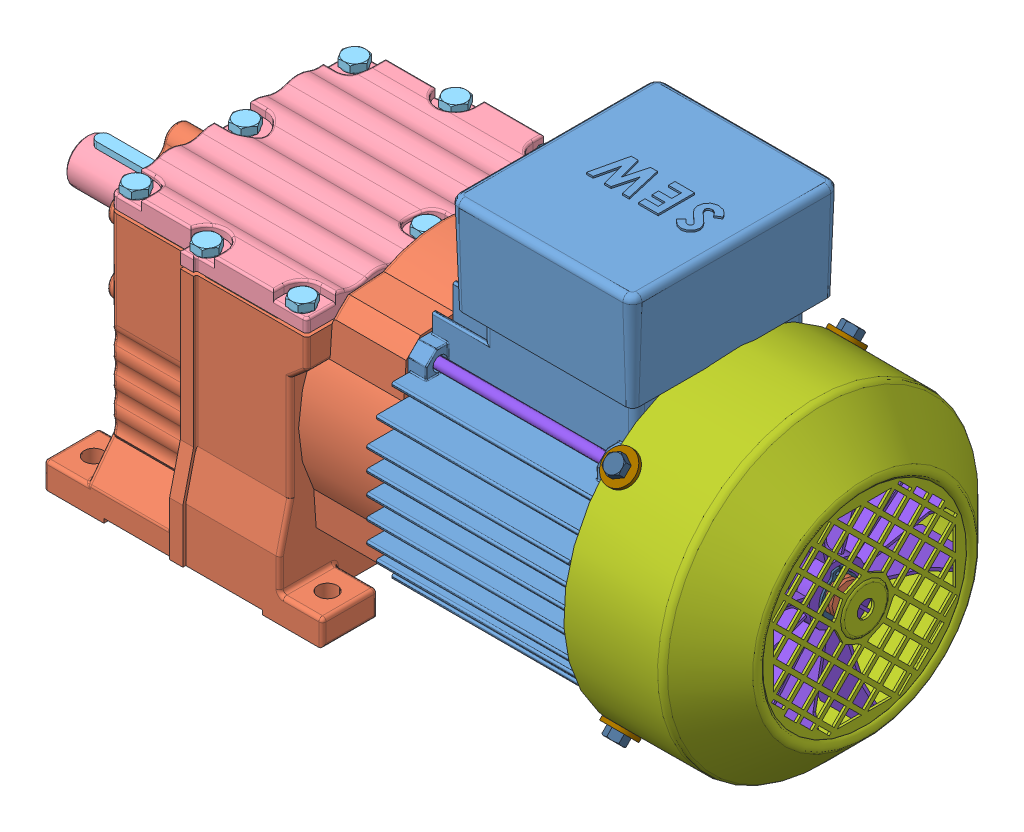
SolidWorks assembly motoreducteur_sew, configuration normale. Lengths in mm.
Overall size (364.24 223.98 208.79).
70 component instances, 46 part files, 12 mates.
Components (placement in the parent):
- bati-1: bati [Défaut] at (-5.3482 -13.3943 0) size (322.68 223.98 208.79)
  - stator-1: stator [Défaut] at origin size (109 189.98 140.8)
  - carter_reducteur-1: carter_reducteur [Défaut] at (-128.4692 42 0) x (0 0 1) z (0 1 0) size (138.68 158.48 134.18)
  - joint plat-1: joint plat [Défaut] at (-128.4692 43.6 0.18) x (0 0 -1) z (0 -1 0) size (123.38 94.6 1.6)
  - couvercle-1: couvercle [Défaut] at (-128.4692 43.6 0) x (0 0 1) z (0 1 0) size (128.68 97.78 10)
  - vis HM6-16-1: vis HM6-16 [Default] at (-122.22 53.6 -51) x (0 -1 0) z (0 0 1) size (20 11.55 10)
  - vis HM6-16-4: vis HM6-16 [Default] at (-122.22 53.6 0) x (0 -1 0) z (0 0 1) size (20 11.55 10)
  - vis HM6-16-5: vis HM6-16 [Default] at (-122.22 53.6 51) x (0 -1 0) z (0 0 1) size (20 11.55 10)
  - vis HM6-16-6: vis HM6-16 [Default] at (-37.62 53.6 58) x (0 -1 0) z (0 0 1) size (20 11.55 10)
  - vis HM6-16-7: vis HM6-16 [Default] at (-37.62 53.6 0) x (0 -1 0) z (0 0 1) size (20 11.55 10)
  - vis HM6-16-8: vis HM6-16 [Default] at (-37.62 53.6 -58) x (0 -1 0) z (0 0 1) size (20 11.55 10)
  - vis HM6-16-9: vis HM6-16 [Default] at (-82.22 53.6 58) x (0 -1 0) z (0 0 1) size (20 11.55 10)
  - vis HM6-16-10: vis HM6-16 [Default] at (-82.22 53.6 -58) x (0 -1 0) z (0 0 1) size (20 11.55 10)
  - flasque-1: flasque [Défaut] at (127.08 0 0) x (-1 0 0) z (0 -0.707107 -0.707107) size (27.7 143 143)
  - carter-1: carter [Défaut] at (166.08 0 0) x (1 0 0) z (0 0.707107 0.707107) size (67.9 147.64 147.64)
  - vis Chc - M5 x 115-15-1: vis Chc - M5 x 115-15 [Default] at (113.58 43.5578 -43.5578) x (-1 0 0) z (0 -0.707107 0.707107) size (118.5 9.24 8)
  - vis Chc - M5 x 115-15-2: vis Chc - M5 x 115-15 [Default] at (113.58 -43.5578 -43.5578) x (-1 0 0) z (0 0.707107 0.707107) size (118.5 9.24 8)
  - vis Chc - M5 x 115-15-3: vis Chc - M5 x 115-15 [Default] at (113.58 -43.5578 43.5578) x (-1 0 0) z (0 0.707107 -0.707107) size (118.5 9.24 8)
  - vis Chc - M5 x 115-15-4: vis Chc - M5 x 115-15 [Default] at (113.58 43.5578 43.5578) x (-1 0 0) z (0 -0.707107 -0.707107) size (118.5 9.24 8)
  - rondelle M5-1: rondelle M5 [Default] at (105.58 52.1986 52.1986) x (0 -0.707107 -0.707107) z (0.685439 -0.514866 0.514866) size (1.75 15 15)
  - vis HM5-6-1: vis HM5-6 [Default] at (105.58 56.1231 56.1231) x (0 -0.707107 -0.707107) z (0.5 -0.612372 0.612372) size (9.8 9.24 8)
  - vis HM5-6-2: vis HM5-6 [Default] at (105.58 -56.1231 56.1231) x (0 0.707107 -0.707107) z (0.5 -0.612372 -0.612372) size (9.8 9.24 8)
  - vis HM5-6-3: vis HM5-6 [Default] at (105.58 -56.1231 -56.1231) x (0 0.707107 0.707107) z (0.5 0.612372 -0.612372) size (9.8 9.24 8)
  - vis HM5-6-4: vis HM5-6 [Default] at (105.58 56.1231 -56.1231) x (0 -0.707107 0.707107) z (0.5 0.612372 0.612372) size (9.8 9.24 8)
  - rondelle M5-2: rondelle M5 [Default] at (105.58 -52.1986 52.1986) x (0 0.707107 -0.707107) z (0.685439 -0.514866 -0.514866) size (1.75 15 15)
  - rondelle M5-3: rondelle M5 [Default] at (105.58 -52.1986 -52.1986) x (0 0.707107 0.707107) z (0.685439 0.514866 -0.514866) size (1.75 15 15)
  - rondelle M5-4: rondelle M5 [Default] at (105.58 52.1986 -52.1986) x (0 -0.707107 0.707107) z (0.685439 0.514866 0.514866) size (1.75 15 15)
  - bouchon visse-1: bouchon visse [Défaut] at (-27.72 -60.575 19.6658) x (0 1 0) z (0.5 0 0.866025) size (12.4 14 14)
  - bouchon visse-2: bouchon visse [Défaut] at (-132.22 26 -43) size (12.4 14 14)
  - bouchon-1: bouchon [Défaut] at (-135.22 -35.5709 20.3891) x (1 0 0) z (0 0.161787 0.986826) size (8 32 32)
  - anneau elastique 47 x 1.75-1: anneau elastique 47 x 1.75 [Default] at (-12.32 0 0) x (0 0 1) z (-1 0 0) size (49.5 48.65 1.75)
  - anneau elastique 42 x 1.75-1: anneau elastique 42 x 1.75 [Default] at (-147.05 0 0) x (0 0 1) z (-1 0 0) size (44.5 43.63 1.75)
  - anneau elastique 32 x 1.2-1: anneau elastique 32 x 1.2 [Default] at (-126.52 -35.5709 20.3891) x (0 0 1) z (-1 0 0) size (33.7 33.12 1.2)
  - joints a levres 25-42-7-1: joints a levres 25-42-7 [Défaut] at (-154.62 0 0) size (7.15 42 42)
  - rondelle elastique-1: rondelle elastique [Défaut] at (115.58 -25.2441 19.8699) x (0 1 0) z (0 0 1) size (39 2.61 39)
  - Joint a levres 17-40-7-1: Joint a levres 17-40-7 [Défaut] at (-28.72 0 0) x (-1 0 0) z (0 -0.924225 -0.381849) size (7 40 40)
  - rondelle d'appui-1: rondelle d'appui [Défaut] at (-28.72 0 0) x (1 0 0) z (0 0.006733 0.999977) size (2.5 46.76 46.76)
- ensemble rotor-2: ensemble rotor [Défaut] at (35.7383 -25.477 0) x (-1 0 0) z (0 0 -1) size (224.99 161.67 158.62)
  - rotor-1: rotor [Défaut] at (-117.0635 12.0827 0) size (224.59 61.49 61.49)
  - roulement 6303Z-1: roulement 6303Z [SKF - 6303 - 8,DE,NC,8_68] at (60.4065 12.0827 0) x (-1 0 0) z (0 0 1) size (14 47 47)
  - roulement 6203DU-1: roulement 6203DU [Default] at (-67.5835 12.0827 0) size (12 40 40)
  - clavette _5_5_18-1: clavette _5_5_18 [Défaut] at (-109.5635 16.5827 -2.5) x (1 0 0) z (0 1 0) size (18 5 5)
  - clavette _2_2_12-1: clavette _2_2_12 [Défaut] at (93.0865 15.8827 -1) x (1 0 0) z (0 1 0) size (12 2 2)
  - pignon entree-1: pignon entree [Défaut] at (105.0865 12.0827 0) x (0 0 -1) z (1 0 0) size (30.84 30.85 16.04)
  - ventilateur-1: ventilateur [Défaut] at (-113.0635 12.0827 0) x (1 0 0) z (0 0.258819 0.965926) size (32 132 132)
  - anneau elastique 10 x 1-1: anneau elastique 10 x 1 [Default] at (106.0865 12.0827 0) x (0 0.030414 0.999537) z (1 0 0) size (12.4 14.94 1)
  - anneau elastique 15 x 1-1: anneau elastique 15 x 1 [Default] at (-113.0635 12.0827 0) x (0 -0.023256 0.99973) z (1 0 0) size (17.51 20.1 1)
  - anneau elastique 17 x 1-1: anneau elastique 17 x 1 [Default] at (68.4065 12.0827 0) x (0 0.021008 0.999779) z (1 0 0) size (19.57 22.3 1)
  - flasque roulement-1: flasque roulement [Défaut] at (53.2065 12.0827 0) x (1 0 0) z (0 0.014788 0.999891) size (2 37 37)
  - deflecteur-1: deflecteur [Défaut] at (84.4065 12.0827 0) x (-1 0 0) z (0 -0.924225 -0.381849) size (3.99 32 32)
  - Joint_Vring_17-1: Joint_Vring_17 [Défaut] at (-92.6935 12.0827 0) x (0 0.691088 0.722771) z (-1 0 0) size (23 23 6.7)
- arbre intermediaire-1: arbre intermediaire [Défaut] at (-97.3682 -48.9652 20.3891) x (0 0 1) z (1 0 0) size (53.96 53.98 80.5)
  - pignon arbre-1: pignon arbre [Défaut] at origin size (14.47 14.51 80.5)
  - roulement 6201-1: roulement 6201 [Default] at (0 0 5) x (0 0 -1) z (1 0 0) size (10 32 32)
  - roulement 6201-2: roulement 6201 [Default] at (0 0 -28.3) x (0 0 1) z (-1 0 0) size (10 32 32)
  - entretoise arbre intermediaire-1: entretoise arbre intermediaire [Défaut] at (0 0 27.98) x (0 0 -1) z (1 0 0) size (17.98 18 18)
  - clavette _4_4_8-1: clavette _4_4_8 [Défaut] at (2 3 29.7) x (0 0 1) z (-1 0 0) size (8 4 4)
  - roue entree-1: roue entree [Défaut] at (0 -41 28.58) x (-1 0 0) z (0 0 -1) size (53.96 53.98 10.07)
  - anneau elastique 11 x 1-1: anneau elastique 11 x 1 [Défaut] at (0 0 37.98) size (13.2 15.53 1)
  - anneau elastique 10 x 1-4: anneau elastique 10 x 1 [Default] at (0 0 -36.5) x (-1 0 0) z (0 0 -1) size (12.4 14.94 1)
  - rondelle d'epaisseur-1: rondelle d'epaisseur [Défaut] at (0 0 -33.3) x (0 0 -1) z (1 0 0) size (2.1 18 18)
- arbre de sortie-1: arbre de sortie [Défaut] at (-137.4702 -17.9077 0) size (118.46 70.14 70.15)
  - arbre de sortie-1: arbre de sortie [Défaut] at (-64.138 4.5134 0) size (118.46 25 25)
  - clavette _6_6_32-1: clavette _6_6_32 [Défaut] at (-56.438 11.0134 -3) x (1 0 0) z (0 1 0) size (32 6 6)
  - roulement 6004-1: roulement 6004 [Default] at (-7.198 4.5134 0) x (-1 0 0) z (0 0 -1) size (12 42 42)
  - entretoise arbre de sortie-1: entretoise arbre de sortie [Défaut] at (-1.198 4.5134 0) size (19.44 25.3 25.3)
  - clavette _6_6_16-1: clavette _6_6_16 [Défaut] at (21.302 -7.4866 -3) size (16 6 6)
  - roue sortie-1: roue sortie [Défaut] at (18.242 45.5134 0) x (0 0 -1) z (-1 0 0) size (70.15 70.14 21.87)
  - roulement 6202-1: roulement 6202 [Default] at (45.602 4.5134 0) x (-1 0 0) z (0 0 -1) size (11 35 35)
  - anneau elastique 15 x 1-1: anneau elastique 15 x 1 [Default] at (52.102 4.5134 0) x (0 0 -1) z (1 0 0) size (17.51 20.1 1)
Mates (geometry in assembly coordinates):
- Coaxiale2: concentric aligned: cylinder of bati-1/carter_reducteur-1
- Coïncidente5: coincident anti-aligned: plane of ?; plane of ?
- Coaxiale3: concentric anti-aligned: unknown of bati-1/carter_reducteur-1
- Coïncidente8: coincident anti-aligned: unknown of bati-1/carter_reducteur-1
- Coaxiale4: concentric aligned: unknown of bati-1/carter_reducteur-1
- Coïncidente9: coincident anti-aligned: unknown of bati-1/carter_reducteur-1
- vue en coupe arbre sortie: parallel aligned: unknown of arbre de sortie-1/clavette _6_6_32-1
- vue en coupe arbre intermediaire: unknown aligned: unknown of arbre intermediaire-1/pignon arbre-1
- vue en coupe rotor: unknown = 170 mm aligned: unknown of ensemble rotor-2/clavette _5_5_18-1
- Esquisse3: unknown = 135 mm: unknown of arbre intermediaire-1/pignon arbre-1; axis of bati-1/bouchon-1
- Esquisse4: unknown: unknown of bati-1/carter_reducteur-1; unknown of bati-1/carter_reducteur-1; unknown of bati-1/carter_reducteur-1
- ecorche3: unknown = 15 mm: unknown of bati-1/carter_reducteur-1
